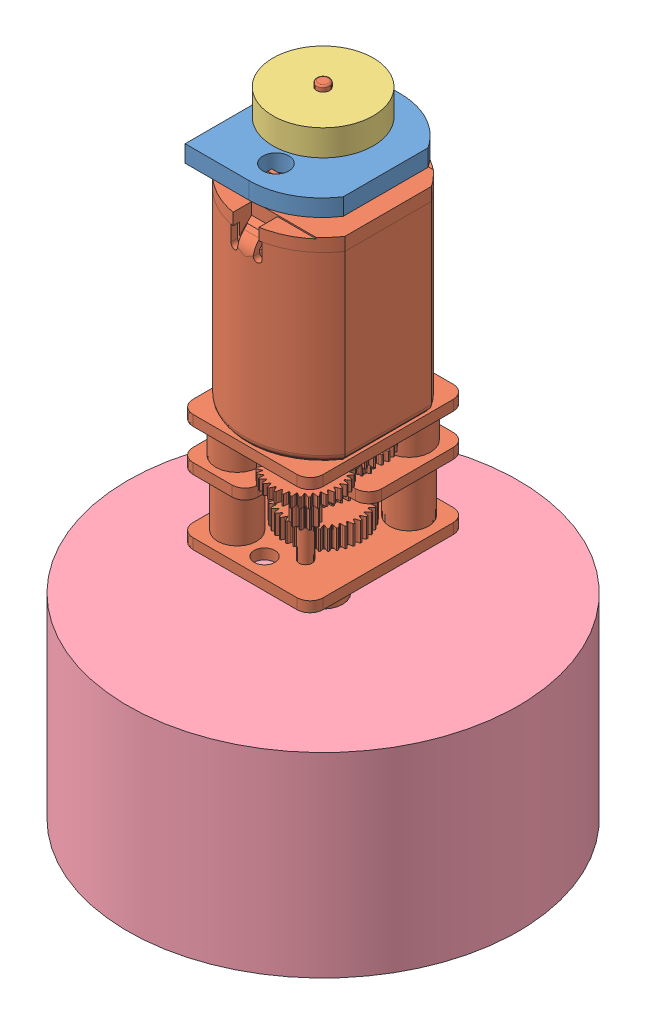
SolidWorks assembly Silnik_enk, configuration Domyślna. Lengths in mm.
Overall size (30.14 49.09 30.14).
5 component instances, 4 part files, 8 mates.
Components (placement in the parent):
- Enkoder_PCB-1: Enkoder_PCB [Domyślna] at (-5.6332 0.2835 8.6889) x (0 0 1) z (0 1 0) size (11.6 9.6 1.3)
- micro-metal-gearmotor-backshaft.step-1: micro-metal-gearmotor-backshaft.step [Domyślna] at (-5.6332 -15.9165 8.6889) x (0 0 1) z (0 -1 0) size (12 10.04 40.2)
- Dysk_pololu-1: Dysk_pololu [Domyślna] at (-5.6332 -14.4184 8.6889) x (0.89461 0 0.446849) z (0 1 0) size (7.7 7.7 2)
- Dysk_pololu-2: Dysk_pololu [Domyślna] at (-5.6332 4.8635 8.6889) x (0.999981 0 -0.006181) z (0 -1 0) size (7.7 7.7 2)
- Kolko-1: Kolko [Domyślna] at (-5.6332 -28.8098 8.6889) x (0.999989 0 -0.004766) z (0 -1 0) size (30 30 15)
Mates (geometry in assembly coordinates):
- Koncentryczne3: concentric anti-aligned: cylinder of Enkoder_PCB-1 through (-5.6332 0.2835 8.6889) axis (0 1 0) radius 1.25; cylinder of micro-metal-gearmotor-backshaft.step-1 through (-5.6332 11.6977 8.6889) axis (0 -1 0) radius 0.5
- Wspólnie2: coincident anti-aligned: plane of Enkoder_PCB-1 through (-5.6332 0.2835 8.6889) normal (0 -1 0); plane of micro-metal-gearmotor-backshaft.step-1 through (-5.6332 0.2835 8.6889) normal (0 1 0)
- Równolegle1: parallel aligned: plane of Enkoder_PCB-1 through (-10.4338 1.5835 8.6889) normal (-1 0 0); plane of micro-metal-gearmotor-backshaft.step-1 through (-10.6322 -0.9165 8.6889) normal (-1 0 0)
- Koncentryczne4: concentric aligned: cylinder of micro-metal-gearmotor-backshaft.step-1 through (-5.6332 11.6977 8.6889) axis (0 -1 0) radius 0.5; cylinder of Dysk_pololu-1 through (-5.6332 -12.4184 8.6889) axis (0 -1 0) radius 0.5
- Prostopadle1: perpendicular: plane of micro-metal-gearmotor-backshaft.step-1 through (-0.6332 -1.9165 8.6889) normal (1 0 0)
- Równolegle2: parallel anti-aligned: plane of Enkoder_PCB-1 through (-5.6332 1.5835 2.8901) normal (0 0 -1)
- Koncentryczne5: concentric anti-aligned: cylinder of micro-metal-gearmotor-backshaft.step-1 through (-5.6332 11.6977 8.6889) axis (0 -1 0) radius 0.5; cylinder of Dysk_pololu-2 through (-5.6332 2.8635 8.6889) axis (0 1 0) radius 0.5
- Koncentryczne6: concentric anti-aligned: cylinder of micro-metal-gearmotor-backshaft.step-1 through (-5.6332 -29.4415 8.6889) axis (0 -1 0) radius 1.5; cylinder of Kolko-1 through (-5.6332 -43.8098 8.6889) axis (0 1 0) radius 1.45
